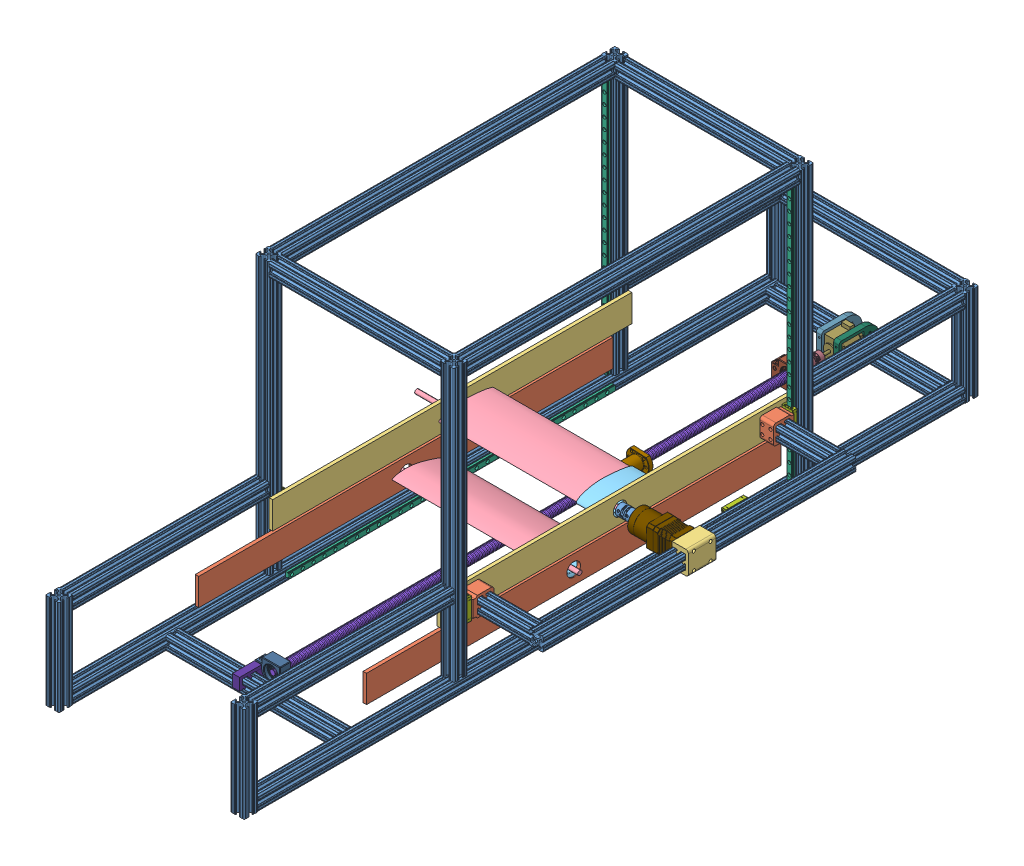
SolidWorks assembly Updated Assembly, configuration Default. Lengths in mm.
Overall size (524.85 538.09 1350.8).
61 component instances, 22 part files, 103 mates.
Components (placement in the parent):
- 47065T121_T-Slotted Framing-2: 47065T121_T-Slotted Framing [1300 mm] at (170.2 12.7 40.4) size (25.4 25.4 1300)
- 47065T121_T-Slotted Framing-3: 47065T121_T-Slotted Framing [1300 mm] at (-170.2 12.7 -40.4) x (-1 0 0) z (0 0 -1) size (25.4 25.4 1300)
- 47065T121_T-Slotted Framing-4: 47065T121_T-Slotted Framing [295mm] at (-157.5 12.7 -637.3) x (0 -1 0) z (1 0 0) size (25.4 25.4 315)
- 47065T121_T-Slotted Framing-5: 47065T121_T-Slotted Framing [175 mm] at (170.2 87.5 662.7) x (1 0 0) z (0 -1 0) size (25.4 25.4 175)
- 47065T121_T-Slotted Framing-6: 47065T121_T-Slotted Framing [175 mm] at (-170.2 87.5 662.7) x (-1 0 0) z (0 1 0) size (25.4 25.4 175)
- 47065T121_T-Slotted Framing-7: 47065T121_T-Slotted Framing [175 mm] at (-170.2 87.5 -662.7) x (-1 0 0) z (0 -1 0) size (25.4 25.4 175)
- 47065T121_T-Slotted Framing-8: 47065T121_T-Slotted Framing [175 mm] at (170.2 87.5 -662.7) x (1 0 0) z (0 1 0) size (25.4 25.4 175)
- Gap Endplate-1: Gap Endplate [Default] at (151.15 70.4 44.0349) x (0 0 -1) z (1 0 0) size (762 50 6.35)
- Stagger Endplate-1: Stagger Endplate [Default] at (151.15 124.5241 -41.19) x (0 0 -1) z (1 0 0) size (660.4 50 6.35)
- 47065T121_T-Slotted Framing-21: 47065T121_T-Slotted Framing [295mm] at (-157.5 162.3 -662.7) x (0 -1 0) z (1 0 0) size (25.4 25.4 315)
- Stagger Endplate-2: Stagger Endplate [Default] at (-157.5 124.5241 -41.19) x (0 0 -1) z (1 0 0) size (660.4 50 6.35)
- Gap Endplate-2: Gap Endplate [Default] at (-157.5 70.4 44.0349) x (0 0 -1) z (1 0 0) size (762 50 6.35)
- Airfoil 2-1: Airfoil 2 [Default] at (-23.65 120.3637 -16.3912) x (0 0.058599 -0.998282) z (1 0 0) size (100.18 14.48 385)
- Airfoil 2-2: Airfoil 2 [Default] at (-23.65 71.3159 69.1635) x (0 -0.143517 -0.989648) z (1 0 0) size (100.18 14.48 385)
- 47065T121_T-Slotted Framing-22: 47065T121_T-Slotted Framing [500 mm] at (170.2 -87.406 -359.29) x (1 0 0) z (0 1 0) size (25.4 25.4 500)
- 47065T121_T-Slotted Framing-28: 47065T121_T-Slotted Framing [500 mm] at (-170.2 635 -359.29) x (-1 0 0) z (0 -1 0) size (25.4 25.4 500)
- 47065T121_T-Slotted Framing-29: 47065T121_T-Slotted Framing [500 mm] at (-170.2 635 276.91) x (-1 0 0) z (0 -1 0) size (25.4 25.4 500)
- 47065T121_T-Slotted Framing-30: 47065T121_T-Slotted Framing [500 mm] at (170.2 635 276.91) x (-1 0 0) z (0 -1 0) size (25.4 25.4 500)
- 47065T121_T-Slotted Framing-31: 47065T121_T-Slotted Framing [295mm] at (-157.5 12.7 466.1) x (0 -1 0) z (1 0 0) size (25.4 25.4 315)
- 47065T121_T-Slotted Framing-32: 47065T121_T-Slotted Framing [560 mm] at (-170.2 512.7 264.21) x (-1 0 0) z (0 0 -1) size (25.4 25.4 610.8)
- 47065T121_T-Slotted Framing-33: 47065T121_T-Slotted Framing [560 mm] at (170.2 512.7 264.21) x (-1 0 0) z (0 0 -1) size (25.4 25.4 610.8)
- 47065T121_T-Slotted Framing-34: 47065T121_T-Slotted Framing [295mm] at (-157.5 509.494 -359.29) x (0 -1 0) z (1 0 0) size (25.4 25.4 315)
- 47065T121_T-Slotted Framing-35: 47065T121_T-Slotted Framing [295mm] at (-157.5 512.7 276.91) x (0 -1 0) z (1 0 0) size (25.4 25.4 315)
- 47065T121_T-Slotted Framing-36: 47065T121_T-Slotted Framing [360.39 mm] at (170.2 162.3 650) x (-1 0 0) z (0 0 -1) size (25.4 25.4 360.39)
- 47065T121_T-Slotted Framing-37: 47065T121_T-Slotted Framing [360.39 mm] at (-170.2 162.3 650) x (-1 0 0) z (0 0 -1) size (25.4 25.4 360.39)
- 47065T121_T-Slotted Framing-38: 47065T121_T-Slotted Framing [278 mm] at (-170.2 162.3 -372) x (-1 0 0) z (0 0 -1) size (25.4 25.4 278)
- 47065T121_T-Slotted Framing-39: 47065T121_T-Slotted Framing [278 mm] at (170.2 162.3 -372) x (-1 0 0) z (0 0 -1) size (25.4 25.4 278)
- Airfoil-2 bottom-1: Airfoil-2 bottom [Default] at (141.15 120.3637 -16.3912) x (0 0.058599 -0.998282) z (1 0 0) size (123.38 36.29 53.26)
- Airfoil-2 bottom-2: Airfoil-2 bottom [Default] at (141.15 71.3159 69.1635) x (0 -0.143517 -0.989648) z (1 0 0) size (123.38 36.29 53.26)
- MGN9-1: MGN9 [По умолчанию] at (154.25 12.7 -341.19) x (0 1 0) z (0 0 1) size (9 6.5 600)
  - v1_MGN9_250-1: v1_MGN9_250 [По умолчанию] at origin size (9 6.5 600)
- MGN9-2: MGN9 [По умолчанию] at (-154.25 12.7 258.81) x (0 1 0) z (0 0 -1) size (9 6.5 600)
  - v1_MGN9_250-1: v1_MGN9_250 [По умолчанию] at origin size (9 6.5 600)
- v1_MGN9_250-1: v1_MGN9_250 [Vertical Rail] at (-170.2 25.4 260.96) x (1 0 0) z (0 1 0) size (9 6.5 474.47)
- v1_MGN9-H-1: v1_MGN9-H [По умолчанию] at (-170.3154 124.5241 258.21) x (1 0 0) z (0 1 0) size (20 8 41.29)
- Ball_screw_Sub_v2-1: Ball_screw_Sub_v2 [Default] at (264.8047 -279.0246 417.4002) x (-0.974812 -0.223029 0) z (0 0 -1) size (68.96 62.55 1139.12)
  - Generic Ballscrew-1: Generic Ballscrew [SFU-1605] at (190.2497 355.7697 977.0002) size (16.19 18.48 1000)
  - Generic Nut-1: Generic Nut [SFU-1204] at (190.2497 355.7697 656.008) x (-0.963177 -0.268868 0) z (0 0 1) size (42 30 36.5)
  - BF12-2: BF12 [Default] at (195.8255 331.3995 -15.9998) x (0.974812 0.223029 0) z (0 0 1) size (60 43 20)
  - BK12-2: BK12 [Default] at (195.8255 331.3995 936.0002) x (0.974812 0.223029 0) z (0 0 1) size (60 46.94 35.34)
  - stepper_cadd_model-2: stepper_cadd_model [Default] at (206.0372 380.9244 1003.0002) x (-0.974812 -0.223029 0) z (0 0 1) size (42 48.5 65)
  - flex coupler_5_to_10-1: flex coupler_5_to_10 [Default] at (190.2497 355.7697 961.0002) x (0.716266 -0.697827 0) z (-0.697827 -0.716266 0) size (18.93 24 18)
  - X_stepper_brack_V1_left-bk12_compensated-1: X_stepper_brack_V1_left-bk12_compensated [47065T413] at (213.5427 348.1194 1054.7002) x (0 0 1) z (-0.974812 -0.223029 0) size (74.4 46.71 10)
  - X_stepper_brack_V1_Right-bk12_compensated-1: X_stepper_brack_V1_Right-bk12_compensated [47065T413] at (172.6006 338.7522 1054.7002) x (0 0 1) z (-0.974812 -0.223029 0) size (74.4 46.71 10.22)
  - 47065T413_T-Slotted Framing-1: 47065T413_T-Slotted Framing [width] at (195.4588 344.253 -49.0198) x (0 0 -1) z (0.974812 0.223029 0) size (25.4 25.4 314.33) (hidden)
  - tslot_to_ballscrew_mirrored-2: tslot_to_ballscrew_mirrored [Default] at (166.5811 324.7086 -30.9998) x (0.974812 0.223029 0) z (0 0 1) size (30 30.65 40.72)
  - tslot_to_ballscrew-3: tslot_to_ballscrew [Default] at (166.5811 324.7086 -30.9998) x (0.974812 0.223029 0) z (0 0 1) size (30 30.65 40.72)
- 17HS15-1684-HG10-1: 17HS15-1684-HG10 [Default] at (278.3 124.5241 -41.19) x (1 0 0) z (0 -1 0) size (109.65 42.3 53.3)
- NEMA17_Coupler-1: NEMA17_Coupler [Default] at (158.5 124.5241 -41.19) x (0 -0.924785 0.380489) z (0 0.380489 0.924785) size (20 26 20)
- 47065T121_T-Slotted Framing-40: 47065T121_T-Slotted Framing [120.8 mm] at (217.9 124.5241 233.51) x (0 0 1) z (-1 0 0) size (25.4 25.4 120.8)
- v1_MGN9_250-2: v1_MGN9_250 [Vertical Rail] at (169.8 25.4 260.96) x (1 0 0) z (0 1 0) size (9 6.5 474.47)
- v1_MGN9-H-2: v1_MGN9-H [По умолчанию] at (169.6846 124.5241 258.21) x (1 0 0) z (0 1 0) size (20 8 41.29)
- v1_MGN9_250-4: v1_MGN9_250 [Vertical Rail] at (-170.2 499.872 -343.34) x (1 0 0) z (0 -1 0) size (9 6.5 474.47)
- v1_MGN9_250-5: v1_MGN9_250 [Vertical Rail] at (169.8 499.872 -343.34) x (1 0 0) z (0 -1 0) size (9 6.5 474.47)
- 47065T121_T-Slotted Framing-41: 47065T121_T-Slotted Framing [120.8 mm] at (217.9 124.5241 -315.89) x (0 0 -1) z (1 0 0) size (25.4 25.4 120.8)
- 47065T121_T-Slotted Framing-43: 47065T121_T-Slotted Framing [574.8] at (291 124.5241 -41.19) x (-1 0 0) z (0 0 -1) size (25.4 25.4 574.8)
- H9_carriage_mount-Gap-1: H9_carriage_mount-Gap [Default] at (170.3154 124.1468 246.21) size (25 36.15 38.4)
- H9_carriage_mount-Gap-2: H9_carriage_mount-Gap [Default] at (169.6846 124.1468 -328.59) x (-1 0 0) z (0 0 -1) size (25 36.15 38.4)
- v1_MGN9-H-3: v1_MGN9-H [По умолчанию] at (169.6846 124.1468 -340.59) x (-1 0 0) z (0 1 0) size (20 8 41.29)
- v1_MGN9-H-4: v1_MGN9-H [По умолчанию] at (151.5 12.8154 -258.1681) x (0 1 0) z (0 0 1) size (20 8 41.29)
- Gap AOA Bracket-1: Gap AOA Bracket [Default] at (303.7 124.5241 -41.19) x (0 0 -1) z (1 0 0) size (50.81 42.3 30.43)
Mates (geometry in assembly coordinates):
- Symmetric4: symmetric aligned: plane of 47065T121_T-Slotted Framing-2 through (163.7836 3.2902 650) normal (0 0 1); plane of 47065T121_T-Slotted Framing-2 through (163.7836 3.2902 -650) normal (0 0 -1)
- Coincident2: coincident anti-aligned: plane of 47065T121_T-Slotted Framing-2 through (160.6496 0 650) normal (0 -1 0)
- Coincident4: coincident anti-aligned: plane of 47065T121_T-Slotted Framing-4 through (157.5 0 -643.6331) normal (0 -1 0)
- Coincident6: coincident aligned: plane of 47065T121_T-Slotted Framing-3 through (-163.7836 3.2902 -650) normal (0 0 -1); plane of 47065T121_T-Slotted Framing-4 through (157.5 19.0331 -650) normal (0 0 -1)
- Coincident9: coincident aligned: plane of 47065T121_T-Slotted Framing-2 through (182.9 19.0331 650) normal (1 0 0); plane of 47065T121_T-Slotted Framing-5 through (182.9 0 669.0331) normal (1 0 0)
- Coincident36: coincident aligned: plane of 47065T121_T-Slotted Framing-7 through (-163.8669 0 -675.4) normal (0 0 -1); plane of 47065T121_T-Slotted Framing-21 through (157.5 168.6331 -675.4) normal (0 0 -1)
- Concentric2: concentric aligned: cylinder of Stagger Endplate-1 through (157.5 124.5241 -41.19) axis (-1 0 0) radius 12.5; cylinder of Airfoil 2-1 through (168.85 124.5241 -41.19) axis (-1 0 0) radius 3.9688
- Concentric3: concentric aligned: cylinder of Gap Endplate-1 through (151.15 70.4 44.0349) axis (1 0 0) radius 12.5; cylinder of Airfoil 2-2 through (-216.15 70.4 44.0349) axis (1 0 0) radius 3.9688
- Distance1: distance = 70 mm aligned: plane of Gap Endplate-1 through (157.5 95.4 425.0349) normal (0 1 0); plane of 47065T121_T-Slotted Framing-2 through (163.8669 25.4 650) normal (0 1 0)
- Coincident43: coincident anti-aligned: plane of 47065T121_T-Slotted Framing-7 through (-157.5 0 -656.3669) normal (1 0 0); plane of 47065T121_T-Slotted Framing-21 through (-157.5 168.7164 -653.2902) normal (-1 0 0)
- Coincident44: coincident anti-aligned: plane of 47065T121_T-Slotted Framing-8 through (157.5 175 -656.3669) normal (-1 0 0); plane of 47065T121_T-Slotted Framing-21 through (157.5 168.7164 -653.2902) normal (1 0 0)
- Coincident48: coincident anti-aligned: plane of 47065T121_T-Slotted Framing-2 through (157.5 22.2504 650) normal (-1 0 0); plane of 47065T121_T-Slotted Framing-4 through (157.5 19.1164 -627.8902) normal (1 0 0)
- Coincident49: coincident anti-aligned: plane of Stagger Endplate-2 through (-151.15 124.5241 -41.19) normal (1 0 0); plane of Airfoil 2-1 through (-151.15 121.5155 -16.8212) normal (-1 0 0)
- Parallel1: parallel aligned: plane of Gap Endplate-1 through (157.5 95.4 425.0349) normal (0 1 0); plane of Stagger Endplate-1 through (157.5 149.5241 289.01) normal (0 1 0)
- Coincident56: coincident anti-aligned: plane of 47065T121_T-Slotted Framing-8 through (157.5 175 -656.3669) normal (-1 0 0); plane of Gap Endplate-1 through (157.5 70.4 44.0349) normal (1 0 0)
- Coincident57: coincident aligned: plane of 47065T121_T-Slotted Framing-2 through (182.9 19.0331 650) normal (1 0 0); plane of 47065T121_T-Slotted Framing-22 through (182.9 522.194 -365.6231) normal (1 0 0)
- Coincident58: coincident anti-aligned: plane of 47065T121_T-Slotted Framing-2 through (163.8669 25.4 650) normal (0 1 0); plane of 47065T121_T-Slotted Framing-22 through (163.7836 25.4 -324.4802) normal (0 -1 0)
- LimitDistance1: limit distance = 85.2249 mm aligned: plane of Gap Endplate-1 through (151.15 70.4 44.0349) normal (0 0 -1); plane of Stagger Endplate-1 through (151.15 124.5241 -41.19) normal (0 0 -1)
- Coincident63: coincident anti-aligned: plane of 47065T121_T-Slotted Framing-3 through (-179.7504 25.4 -650) normal (0 1 0); plane of 47065T121_T-Slotted Framing-28 through (-163.7836 25.4 -349.8802) normal (0 -1 0)
- Coincident64: coincident aligned: plane of 47065T121_T-Slotted Framing-3 through (-157.5 22.2504 -650) normal (1 0 0); plane of 47065T121_T-Slotted Framing-28 through (-157.5 25.4 -352.9569) normal (1 0 0)
- Coincident65: coincident aligned: plane of 47065T121_T-Slotted Framing-22 through (163.8669 522.194 -371.99) normal (0 0 -1); plane of 47065T121_T-Slotted Framing-28 through (-163.8669 25.4 -371.99) normal (0 0 -1)
- Coincident66: coincident aligned: plane of 47065T121_T-Slotted Framing-28 through (-182.9 25.4 -349.7396) normal (-1 0 0); plane of 47065T121_T-Slotted Framing-29 through (-182.9 25.4 270.5769) normal (-1 0 0)
- Coincident67: coincident anti-aligned: plane of 47065T121_T-Slotted Framing-3 through (-163.8669 25.4 -650) normal (0 1 0); plane of 47065T121_T-Slotted Framing-29 through (-163.7836 25.4 286.3198) normal (0 -1 0)
- Coincident68: coincident anti-aligned: plane of 47065T121_T-Slotted Framing-2 through (163.8669 25.4 650) normal (0 1 0); plane of 47065T121_T-Slotted Framing-30 through (176.6164 25.4 286.3198) normal (0 -1 0)
- Coincident69: coincident aligned: plane of 47065T121_T-Slotted Framing-2 through (182.9 19.0331 650) normal (1 0 0); plane of 47065T121_T-Slotted Framing-30 through (182.9 25.4 267.3596) normal (1 0 0)
- Coincident70: coincident aligned: plane of 47065T121_T-Slotted Framing-29 through (-176.5331 25.4 289.61) normal (0 0 1); plane of 47065T121_T-Slotted Framing-30 through (163.8669 25.4 289.61) normal (0 0 1)
- Coincident71: coincident anti-aligned: plane of Stagger Endplate-1 through (157.5 124.5241 -41.19) normal (1 0 0); plane of 47065T121_T-Slotted Framing-22 through (157.5 522.194 -352.9569) normal (-1 0 0)
- Coincident72: coincident aligned: plane of 47065T121_T-Slotted Framing-3 through (-179.7504 25.4 -650) normal (0 1 0); plane of 47065T121_T-Slotted Framing-31 through (157.5 25.4 472.4331) normal (0 1 0)
- Coincident73: coincident anti-aligned: plane of 47065T121_T-Slotted Framing-2 through (157.5 22.2504 650) normal (-1 0 0); plane of 47065T121_T-Slotted Framing-31 through (157.5 19.1164 475.5098) normal (1 0 0)
- Coincident75: coincident anti-aligned: plane of 47065T121_T-Slotted Framing-29 through (-163.8669 25.4 264.21) normal (0 0 -1); plane of 47065T121_T-Slotted Framing-32 through (-163.7836 503.2902 264.21) normal (0 0 1)
- Coincident76: coincident aligned: plane of 47065T121_T-Slotted Framing-29 through (-163.7836 525.4 260.9198) normal (0 1 0); plane of 47065T121_T-Slotted Framing-32 through (-163.8669 525.4 -321.19) normal (0 1 0)
- Coincident77: coincident aligned: plane of 47065T121_T-Slotted Framing-29 through (-157.5 25.4 283.2431) normal (1 0 0); plane of 47065T121_T-Slotted Framing-32 through (-157.5 522.2504 -346.59) normal (1 0 0)
- Coincident78: coincident anti-aligned: plane of 47065T121_T-Slotted Framing-28 through (-160.6496 25.4 -346.59) normal (0 0 1); plane of 47065T121_T-Slotted Framing-32 through (-163.7836 503.2902 -346.59) normal (0 0 -1)
- Coincident79: coincident anti-aligned: plane of Gap Endplate-2 through (-151.15 70.4 44.0349) normal (1 0 0); plane of Airfoil 2-2 through (-151.15 72.3575 68.5105) normal (-1 0 0)
- Coincident82: coincident anti-aligned: plane of 47065T121_T-Slotted Framing-22 through (157.5 522.194 -352.9569) normal (-1 0 0); plane of 47065T121_T-Slotted Framing-34 through (157.5 515.9104 -349.8802) normal (1 0 0)
- Coincident83: coincident aligned: plane of 47065T121_T-Slotted Framing-22 through (179.7504 522.194 -371.99) normal (0 0 -1); plane of 47065T121_T-Slotted Framing-34 through (157.5 515.8271 -371.99) normal (0 0 -1)
- Coincident84: coincident aligned: plane of 47065T121_T-Slotted Framing-22 through (163.7836 522.194 -349.8802) normal (0 1 0); plane of 47065T121_T-Slotted Framing-34 through (157.5 522.194 -368.8404) normal (0 1 0)
- Coincident86: coincident anti-aligned: plane of 47065T121_T-Slotted Framing-30 through (157.5 25.4 286.4604) normal (-1 0 0); plane of 47065T121_T-Slotted Framing-35 through (157.5 519.1164 286.3198) normal (1 0 0)
- Coincident87: coincident aligned: plane of 47065T121_T-Slotted Framing-30 through (163.8669 25.4 289.61) normal (0 0 1); plane of 47065T121_T-Slotted Framing-35 through (157.5 522.2504 289.61) normal (0 0 1)
- Coincident88: coincident aligned: plane of 47065T121_T-Slotted Framing-30 through (176.6164 525.4 260.9198) normal (0 1 0); plane of 47065T121_T-Slotted Framing-35 through (157.5 525.4 241.9596) normal (0 1 0)
- Coincident90: coincident aligned: plane of 47065T121_T-Slotted Framing-5 through (182.9 0 653.1496) normal (1 0 0); plane of 47065T121_T-Slotted Framing-36 through (182.9 171.8504 289.61) normal (1 0 0)
- Coincident94: coincident aligned: plane of 47065T121_T-Slotted Framing-6 through (-182.9 175 669.0331) normal (-1 0 0); plane of 47065T121_T-Slotted Framing-37 through (-182.9 168.6331 289.61) normal (-1 0 0)
- Coincident96: coincident aligned: plane of 47065T121_T-Slotted Framing-7 through (-182.9 0 -653.1496) normal (-1 0 0); plane of 47065T121_T-Slotted Framing-38 through (-182.9 168.6331 -650) normal (-1 0 0)
- Coincident100: coincident aligned: plane of 47065T121_T-Slotted Framing-8 through (182.9 175 -653.1496) normal (1 0 0); plane of 47065T121_T-Slotted Framing-39 through (182.9 171.8504 -650) normal (1 0 0)
- LimitDistance2: limit distance = 4.1241 mm anti-aligned: plane of Stagger Endplate-1 through (157.5 99.5241 289.01) normal (0 -1 0); plane of Gap Endplate-1 through (157.5 95.4 425.0349) normal (0 1 0)
- Concentric4: concentric anti-aligned: cylinder of Airfoil 2-1 through (168.85 124.5241 -41.19) axis (-1 0 0) radius 3.9688; cylinder of Airfoil-2 bottom-1 through (141.15 124.5241 -41.19) axis (1 0 0) radius 14
- Coincident101: coincident anti-aligned: plane of Airfoil 2-1 through (103.85 121.5155 -16.8212) normal (1 0 0); plane of Airfoil-2 bottom-1 through (103.85 122.6132 -15.1494) normal (-1 0 0)
- Concentric5: concentric anti-aligned: cylinder of Airfoil 2-2 through (168.85 70.4 44.0349) axis (-1 0 0) radius 3.9688; cylinder of Airfoil-2 bottom-2 through (141.15 70.4 44.0349) axis (1 0 0) radius 14
- Coincident102: coincident anti-aligned: plane of Airfoil 2-2 through (103.85 72.3575 68.5105) normal (1 0 0); plane of Airfoil-2 bottom-2 through (103.85 73.7692 69.9272) normal (-1 0 0)
- Parallel2: parallel aligned: plane of Airfoil 2-1 through (-23.65 120.3637 -16.3912) normal (0 0.058599 -0.998282); plane of Airfoil-2 bottom-1 through (141.15 120.3637 -16.3912) normal (0 0.058599 -0.998282)
- Parallel3: parallel aligned: plane of Airfoil 2-2 through (-23.65 71.3159 69.1635) normal (0 -0.143517 -0.989648); plane of Airfoil-2 bottom-2 through (141.15 71.3159 69.1635) normal (0 -0.143517 -0.989648)
- Coincident103: coincident anti-aligned: plane of 47065T121_T-Slotted Framing-2 through (157.5 22.2504 650) normal (-1 0 0); plane of MGN9-1/v1_MGN9_250-1 through (157.5 8.2 258.81) normal (1 0 0)
- Width3: width aligned: plane of 47065T121_T-Slotted Framing-2 through (163.8669 25.4 650) normal (0 1 0); plane of 47065T121_T-Slotted Framing-2 through (160.6496 0 650) normal (0 -1 0); plane of MGN9-1/v1_MGN9_250-1 through (157.5 17.2 258.81) normal (0 1 0); plane of MGN9-1/v1_MGN9_250-1 through (157.5 8.2 258.81) normal (0 -1 0)
- Coincident104: coincident anti-aligned: plane of 47065T121_T-Slotted Framing-29 through (-163.8669 25.4 264.21) normal (0 0 -1); plane of v1_MGN9_250-1 through (-174.7 625.4 264.21) normal (0 0 1)
- Parallel4: parallel anti-aligned: plane of 47065T121_T-Slotted Framing-32 through (-179.7504 525.4 -346.59) normal (0 1 0); plane of v1_MGN9_250-1 through (-174.7 25.4 259.71) normal (0 -1 0)
- Coincident105: coincident anti-aligned: plane of 47065T121_T-Slotted Framing-3 through (-163.8669 25.4 -650) normal (0 1 0); plane of v1_MGN9_250-1 through (-174.7 25.4 259.71) normal (0 -1 0)
- Coincident106: coincident anti-aligned: plane of v1_MGN9_250-1 through (-174.7 625.4 257.71) normal (0 0 -1); plane of v1_MGN9-H-1 through (-170.3154 139.4741 257.71) normal (0 0 1)
- Parallel5: parallel anti-aligned: plane of v1_MGN9_250-1 through (-174.7 625.4 264.21) normal (-1 0 0); plane of v1_MGN9-H-1 through (-160.3154 139.4741 258.21) normal (1 0 0)
- Coincident107: coincident anti-aligned: plane of v1_MGN9_250-1 through (-173.4351 625.4 260.062) normal (-1 0 0); plane of v1_MGN9-H-1 through (-173.4351 144.4741 260.0081) normal (1 0 0)
- Width4: width aligned: plane of 47065T121_T-Slotted Framing-29 through (-182.9 25.4 270.5769) normal (-1 0 0); plane of 47065T121_T-Slotted Framing-29 through (-157.5 25.4 267.3596) normal (1 0 0); plane of v1_MGN9_250-1 through (-174.7 625.4 264.21) normal (-1 0 0); plane of v1_MGN9_250-1 through (-165.7 625.4 264.21) normal (1 0 0)
- Width5: width aligned: plane of 47065T121_T-Slotted Framing-22 through (163.8669 522.194 -371.99) normal (0 0 -1); plane of 47065T121_T-Slotted Framing-30 through (163.8669 25.4 289.61) normal (0 0 1); plane of MGN9-1/v1_MGN9_250-1 through (153 8.2 -341.19) normal (0 0 -1); plane of MGN9-1/v1_MGN9_250-1 through (153 8.2 258.81) normal (0 0 1)
- Concentric6: concentric aligned: cylinder of 47065T121_T-Slotted Framing-4 through (157.5 23.2918 -647.8918) axis (-1 0 0) radius 2.1082; cylinder of Ball_screw_Sub_v2-1/X_stepper_brack_V1_left-bk12_compensated-1 through (-11 23.2918 -647.8918) axis (-1 0 0) radius 2.4282
- Parallel6: parallel aligned: plane of 47065T121_T-Slotted Framing-4 through (157.5 25.4 -630.9669) normal (0 1 0); plane of Ball_screw_Sub_v2-1/X_stepper_brack_V1_left-bk12_compensated-1 through (-11 51.47 -655) normal (0 1 0)
- Width6: width anti-aligned: plane of 47065T121_T-Slotted Framing-2 through (157.5 22.2504 650) normal (-1 0 0); plane of 47065T121_T-Slotted Framing-3 through (-157.5 22.2504 -650) normal (1 0 0); plane of Ball_screw_Sub_v2-1/stepper_cadd_model-2 through (21 40.8527 -590.1) normal (1 0 0); plane of Ball_screw_Sub_v2-1/stepper_cadd_model-2 through (-21 40.8527 -590.1) normal (-1 0 0)
- Parallel7: parallel aligned: plane of 47065T121_T-Slotted Framing-2 through (163.8669 25.4 650) normal (0 1 0); plane of Ball_screw_Sub_v2-1/tslot_to_ballscrew_mirrored-2 through (-30 31.0042 448.4) normal (0 1 0)
- Coincident110: coincident anti-aligned: plane of 47065T121_T-Slotted Framing-31 through (157.5 19.0331 453.4) normal (0 0 -1); plane of Ball_screw_Sub_v2-1/tslot_to_ballscrew-3 through (0 25.3527 453.4) normal (0 0 1)
- Concentric7: concentric anti-aligned: cylinder of Airfoil 2-1 through (168.85 124.5241 -41.19) axis (-1 0 0) radius 3.9688; cylinder of 17HS15-1684-HG10-1 through (168.85 124.5241 -41.19) axis (1 0 0) radius 4
- Concentric8: concentric anti-aligned: cylinder of 17HS15-1684-HG10-1 through (168.85 124.5241 -41.19) axis (1 0 0) radius 4; cylinder of NEMA17_Coupler-1 through (158.5 124.5241 -41.19) axis (-1 0 0) radius 4.025
- Distance2: distance = 1 mm anti-aligned: plane of NEMA17_Coupler-1 through (158.5 121.9624 -40.136) normal (-1 0 0); plane of Stagger Endplate-1 through (157.5 124.5241 -41.19) normal (1 0 0)
- Parallel8: parallel anti-aligned: plane of 47065T121_T-Slotted Framing-2 through (176.5331 0 650) normal (0 -1 0); plane of 17HS15-1684-HG10-1 through (269.3 145.6741 -62.34) normal (0 1 0)
- Coincident113: coincident anti-aligned: plane of Airfoil 2-1 through (168.85 124.5241 -41.19) normal (1 0 0); plane of 17HS15-1684-HG10-1 through (168.85 124.5241 -41.19) normal (-1 0 0)
- Coincident114: coincident anti-aligned: plane of Stagger Endplate-1 through (157.5 124.5241 -41.19) normal (1 0 0); plane of 47065T121_T-Slotted Framing-40 through (157.5 115.1143 227.0936) normal (-1 0 0)
- Width7: width aligned: plane of Stagger Endplate-1 through (157.5 149.5241 289.01) normal (0 1 0); plane of 47065T121_T-Slotted Framing-40 through (157.5 99.5241 289.01) normal (0 -1 0); plane of Stagger Endplate-1 through (157.5 137.2241 227.1769) normal (0 1 0); plane of 47065T121_T-Slotted Framing-40 through (157.5 111.8241 223.9596) normal (0 -1 0)
- Coincident116: coincident aligned: plane of 47065T121_T-Slotted Framing-2 through (176.5331 0 650) normal (0 -1 0); plane of 47065T121_T-Slotted Framing-5 through (163.7836 0 653.2902) normal (0 -1 0)
- Coincident117: coincident anti-aligned: plane of 47065T121_T-Slotted Framing-2 through (163.7836 3.2902 650) normal (0 0 1); plane of 47065T121_T-Slotted Framing-5 through (176.5331 0 650) normal (0 0 -1)
- Distance3: distance = 8 mm anti-aligned: plane of 47065T121_T-Slotted Framing-40 through (157.5 130.8572 246.21) normal (0 0 1); plane of v1_MGN9-H-2 through (169.6846 139.4741 254.21) normal (0 0 -1)
- Width8: width aligned: plane of 47065T121_T-Slotted Framing-29 through (-160.6496 25.4 289.61) normal (0 0 1); plane of 47065T121_T-Slotted Framing-28 through (-163.8669 25.4 -371.99) normal (0 0 -1); plane of Stagger Endplate-2 through (-151.15 99.5241 289.01) normal (0 0 1); plane of Stagger Endplate-2 through (-151.15 99.5241 -371.39) normal (0 0 -1)
- Coincident121: coincident anti-aligned: plane of 47065T121_T-Slotted Framing-6 through (-160.6496 175 650) normal (0 0 -1); plane of 47065T121_T-Slotted Framing-37 through (-163.7836 152.8902 650) normal (0 0 1)
- Coincident122: coincident aligned: plane of 47065T121_T-Slotted Framing-6 through (-163.7836 175 653.2902) normal (0 1 0); plane of 47065T121_T-Slotted Framing-37 through (-179.7504 175 289.61) normal (0 1 0)
- Coincident123: coincident anti-aligned: plane of 47065T121_T-Slotted Framing-5 through (176.5331 0 650) normal (0 0 -1); plane of 47065T121_T-Slotted Framing-36 through (176.6164 152.8902 650) normal (0 0 1)
- Coincident125: coincident aligned: plane of 47065T121_T-Slotted Framing-5 through (163.7836 175 653.2902) normal (0 1 0); plane of 47065T121_T-Slotted Framing-36 through (160.6496 175 289.61) normal (0 1 0)
- Coincident126: coincident anti-aligned: plane of 47065T121_T-Slotted Framing-30 through (163.8669 25.4 289.61) normal (0 0 1); plane of 47065T121_T-Slotted Framing-36 through (176.6164 152.8902 289.61) normal (0 0 -1)
- Coincident127: coincident anti-aligned: plane of 47065T121_T-Slotted Framing-8 through (160.6496 175 -650) normal (0 0 1); plane of 47065T121_T-Slotted Framing-39 through (176.6164 152.8902 -650) normal (0 0 -1)
- Coincident128: coincident aligned: plane of 47065T121_T-Slotted Framing-8 through (163.7836 175 -653.2902) normal (0 1 0); plane of 47065T121_T-Slotted Framing-39 through (160.6496 175 -650) normal (0 1 0)
- Coincident129: coincident aligned: plane of 47065T121_T-Slotted Framing-8 through (163.7836 175 -653.2902) normal (0 1 0); plane of 47065T121_T-Slotted Framing-21 through (157.5 175 -672.2504) normal (0 1 0)
- Coincident130: coincident anti-aligned: plane of 47065T121_T-Slotted Framing-7 through (-176.5331 0 -650) normal (0 0 1); plane of 47065T121_T-Slotted Framing-38 through (-163.7836 152.8902 -650) normal (0 0 -1)
- Coincident131: coincident aligned: plane of 47065T121_T-Slotted Framing-7 through (-163.7836 175 -653.2902) normal (0 1 0); plane of 47065T121_T-Slotted Framing-38 through (-179.7504 175 -650) normal (0 1 0)
- Width9: width aligned: plane of v1_MGN9-H-2 through (174.1846 144.4741 259.71) normal (0 1 0); plane of v1_MGN9-H-2 through (174.1846 104.5741 259.71) normal (0 -1 0); plane of 47065T121_T-Slotted Framing-40 through (157.5 137.2241 243.0604) normal (0 1 0); plane of 47065T121_T-Slotted Framing-40 through (157.5 111.8241 239.8431) normal (0 -1 0)
- Coincident132: coincident aligned: plane of 47065T121_T-Slotted Framing-40 through (157.5 130.8572 246.21) normal (0 0 1); plane of 47065T121_T-Slotted Framing-43 through (297.4164 115.1143 246.21) normal (0 0 1)
- Coincident133: coincident aligned: plane of 47065T121_T-Slotted Framing-41 through (278.3 137.2241 -309.5569) normal (0 1 0); plane of 47065T121_T-Slotted Framing-43 through (297.3331 137.2241 -328.59) normal (0 1 0)
- Coincident134: coincident anti-aligned: plane of 47065T121_T-Slotted Framing-41 through (278.3 115.1143 -309.4736) normal (1 0 0); plane of 47065T121_T-Slotted Framing-43 through (278.3 130.8572 -328.59) normal (-1 0 0)
- Coincident135: coincident anti-aligned: plane of v1_MGN9-H-2 through (169.6846 139.4741 254.21) normal (0 0 -1); plane of H9_carriage_mount-Gap-1 through (170.3154 124.1468 254.21) normal (0 0 1)
- Width10: width aligned: plane of H9_carriage_mount-Gap-1 through (230.0567 106.4468 246.21) normal (0 -1 0); plane of 47065T121_T-Slotted Framing-40 through (230.0567 142.6013 246.21) normal (0 1 0); plane of H9_carriage_mount-Gap-1 through (157.5 111.8241 239.8431) normal (0 -1 0); plane of 47065T121_T-Slotted Framing-40 through (157.5 137.2241 227.1769) normal (0 1 0)
- Coincident136: coincident anti-aligned: plane of Stagger Endplate-1 through (157.5 124.5241 -41.19) normal (1 0 0); plane of H9_carriage_mount-Gap-1 through (157.5 109.5741 251.21) normal (-1 0 0)
- Coincident137: coincident anti-aligned: plane of v1_MGN9_250-5 through (165.3 -100.128 -340.09) normal (0 0 1); plane of v1_MGN9-H-3 through (174.1846 144.0968 -340.09) normal (0 0 -1)
- Parallel9: parallel aligned: plane of v1_MGN9_250-5 through (174.3 -100.128 -346.59) normal (1 0 0); plane of v1_MGN9-H-3 through (179.6846 139.0968 -340.59) normal (1 0 0)
- Coincident138: coincident anti-aligned: plane of v1_MGN9_250-5 through (166.5649 -100.128 -342.442) normal (-1 0 0); plane of v1_MGN9-H-3 through (166.5649 144.0968 -342.3881) normal (1 0 0)
- Concentric12: concentric anti-aligned: cylinder of H9_carriage_mount-Gap-2 through (177.1846 132.1468 -298.19) axis (0 0 -1) radius 2.9; cylinder of v1_MGN9-H-3 through (177.1846 132.1468 -339.59) axis (0 0 1) radius 1.5
- Coincident139: coincident anti-aligned: plane of MGN9-1/v1_MGN9_250-1 through (153.352 15.9351 258.81) normal (0 1 0); plane of v1_MGN9-H-4 through (153.2981 15.9351 -238.2181) normal (0 -1 0)
- Coincident140: coincident anti-aligned: plane of MGN9-1/v1_MGN9_250-1 through (151 8.2 258.81) normal (-1 0 0); plane of v1_MGN9-H-4 through (151 8.3154 -239.1181) normal (1 0 0)
- Concentric14: concentric anti-aligned: circle of 17HS15-1684-HG10-1; cylinder of Gap AOA Bracket-1 through (308.7 140.0241 -25.69) axis (-1 0 0) radius 2.9
- Concentric15: concentric anti-aligned: circle of 17HS15-1684-HG10-1; cylinder of Gap AOA Bracket-1 through (308.7 140.0241 -56.69) axis (-1 0 0) radius 2.9
- Coincident142: coincident anti-aligned: plane of 47065T121_T-Slotted Framing-43 through (303.7 134.0745 -328.59) normal (1 0 0); plane of Gap AOA Bracket-1 through (303.7 124.5241 -41.19) normal (-1 0 0)
